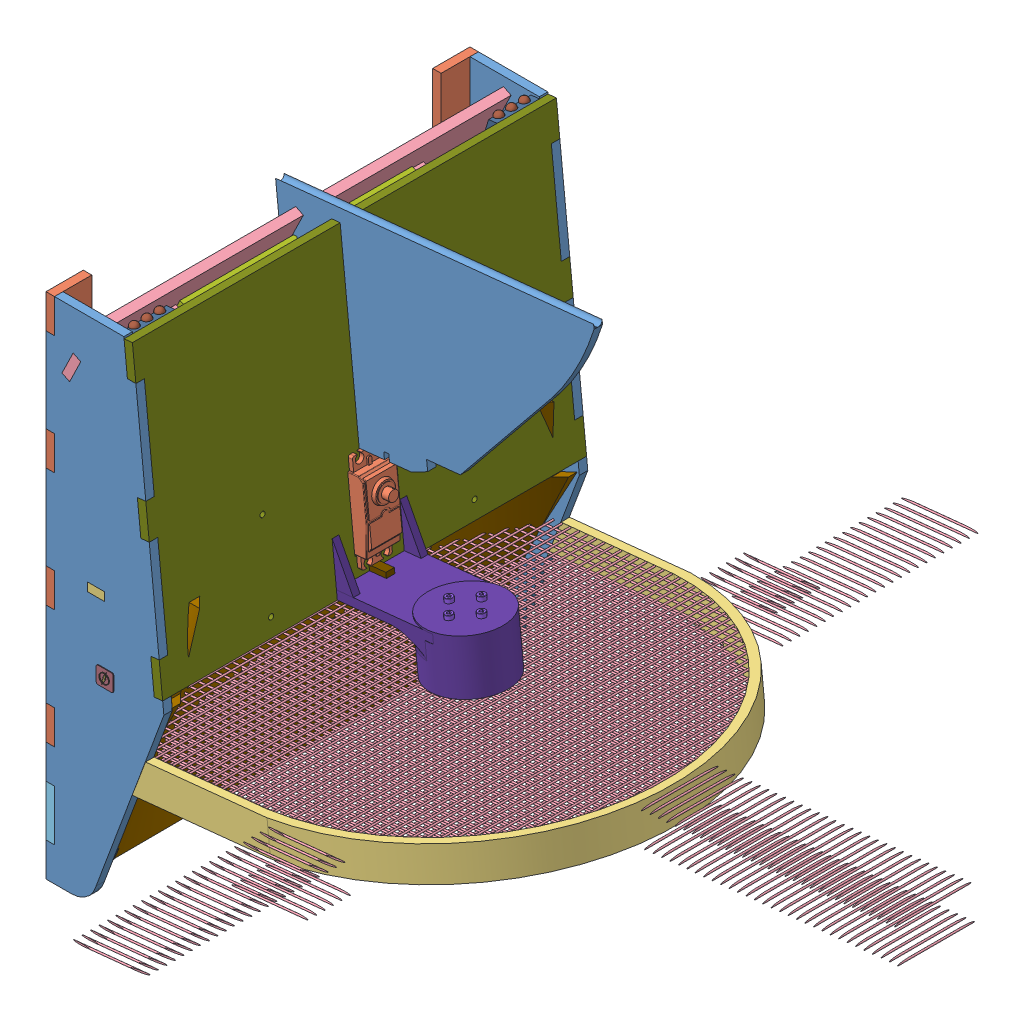
SolidWorks assembly AssStructSimu, configuration Défaut. Lengths in mm. (continued)
Components (placement in the parent): (continued)
- AssCarte-1: AssCarte [Défaut] at (38.0121 147.1029 290.772) x (-0.101852 0.9948 0) z (0.9948 0.101852 0) size (66.52 130.57 98.72) (hidden) (continued)
  - carte_onduleur_v3-1: carte_onduleur_v3 [Défaut] at (-131.8199 12.0892 20.7912) size (66.52 130.57 82.34) (continued)
    - CARTE_CMD-1: CARTE_CMD [Défaut] at (25 57.2 0.803) size (60.1 130 26.71) (continued)
      - Open CASCADE STEP translator 6.8 1.20.1-1: Open CASCADE STEP translator 6.8 1.20.1 [Défaut] at origin size (60.1 130 26.71) (continued)
        - Body_1_4-1: Body_1_4 [Défaut] at (-55 5 12) size (60.1 130 26.71) (continued)
          - 175-1: 175 [Défaut] at (10 -21.7 0.803) x (0 -1 0) z (0 0 1) size (15 25.4 12.78) (continued)
            - =_[0_1_1_72]-1: =_[0_1_1_72] [Défaut] at origin size (15 25.4 12.78) (continued)
              - 173-1: 173 [Défaut] at (-1.4 -1 12) x (-1 0 0) z (0 1 0) size (15 12.78 25.4) (continued)
                - hole_plating_20-20: hole_plating_20 [Défaut] at (-1.5 -1.58 23.93) size (1.5 0.01 1.5)
                - Pin_Header_1x10_TH_Pitch_2.54mm_1-1: Pin_Header_1x10_TH_Pitch_2.54mm_1 [Défaut] at (-1.5 -1.5786 23.93) x (0 0 -1) z (0 -1 0) size (25.4 2.54 12.7)
                  - 124-1: 124 [Défaut] at origin size (25.4 2.54 2.8)
                    - =_[0_1_1_77]-1: =_[0_1_1_77] [Défaut] at origin
                    - =_[0_1_1_79]-1: =_[0_1_1_79] [Défaut] at origin
                    - =_[0_1_1_80]-1: =_[0_1_1_80] [Défaut] at origin
                    - =_[0_1_1_81]-1: =_[0_1_1_81] [Défaut] at origin
                    - =_[0_1_1_82]-1: =_[0_1_1_82] [Défaut] at origin
                    - =_[0_1_1_83]-1: =_[0_1_1_83] [Défaut] at origin
                    - =_[0_1_1_84]-1: =_[0_1_1_84] [Défaut] at origin
                    - =_[0_1_1_85]-1: =_[0_1_1_85] [Défaut] at origin
                    - =_[0_1_1_86]-1: =_[0_1_1_86] [Défaut] at origin
                    - =_[0_1_1_87]-1: =_[0_1_1_87] [Défaut] at origin
                  - 135-1: 135 [Défaut] at origin size (23.49 0.63 12.7)
                    - =_[0_1_1_88]-1: =_[0_1_1_88] [Défaut] at origin size (0.63 0.63 12.7)
                    - =_[0_1_1_90]-1: =_[0_1_1_90] [Défaut] at origin size (0.63 0.63 12.7)
                    - =_[0_1_1_91]-1: =_[0_1_1_91] [Défaut] at origin size (0.63 0.63 12.7)
                    - =_[0_1_1_92]-1: =_[0_1_1_92] [Défaut] at origin size (0.63 0.63 12.7)
                    - =_[0_1_1_93]-1: =_[0_1_1_93] [Défaut] at origin size (0.63 0.63 12.7)
                    - =_[0_1_1_94]-1: =_[0_1_1_94] [Défaut] at origin size (0.63 0.63 12.7)
                    - =_[0_1_1_95]-1: =_[0_1_1_95] [Défaut] at origin size (0.63 0.63 12.7)
                    - =_[0_1_1_96]-1: =_[0_1_1_96] [Défaut] at origin size (0.63 0.63 12.7)
                    - =_[0_1_1_97]-1: =_[0_1_1_97] [Défaut] at origin size (0.63 0.63 12.7)
                    - =_[0_1_1_98]-1: =_[0_1_1_98] [Défaut] at origin size (0.63 0.63 12.7)
                - MPU-9250_1-1: MPU-9250_1 [Défaut] at (-8 0.05 12.5) x (-1 0 0) z (0 1 0) size (3 3 1.05)
                - tantalum_10uF_1-1: tantalum_10uF_1 [Défaut] at (-13.167 0.1 10.9372) x (0 0 1) z (0 1 0)
                - SOT23_5_1-1: SOT23_5_1 [Défaut] at (-7.475 -0.0136 21) x (0 0 1) z (0 1 0) size (3 3.2 0.92)
                - RESC-0603_5-1: RESC-0603_5 [Défaut] at (-6.85 0 7.45) x (1 0 0) z (0 1 0) size (1.7 0.9 0.55)
                  - 143-1: 143 [Défaut] at origin size (1.7 0.9 0.55)
                    - =_[0_1_1_103]-1: =_[0_1_1_103] [Défaut] at origin size (0.4 0.9 0.53)
                    - =_[0_1_1_105]-1: =_[0_1_1_105] [Défaut] at origin size (0.4 0.9 0.53)
                    - =_[0_1_1_106]-1: =_[0_1_1_106] [Défaut] at origin size (1.64 0.9 0.52)
                  - 152-1: 152 [Défaut] at origin
                    - =_[0_1_1_107]-1: =_[0_1_1_107] [Défaut] at origin
                    - =_[0_1_1_109]-1: =_[0_1_1_109] [Défaut] at origin
                    - =_[0_1_1_110]-1: =_[0_1_1_110] [Défaut] at origin
                    - =_[0_1_1_111]-1: =_[0_1_1_111] [Défaut] at origin
                    - =_[0_1_1_112]-1: =_[0_1_1_112] [Défaut] at origin
                    - =_[0_1_1_113]-1: =_[0_1_1_113] [Défaut] at origin
                    - =_[0_1_1_114]-1: =_[0_1_1_114] [Défaut] at origin
                    - =_[0_1_1_115]-1: =_[0_1_1_115] [Défaut] at origin
                - RESC-0603_5-2: RESC-0603_5 [Défaut] at (-9.85 0 16.05) x (1 0 0) z (0 1 0) size (1.7 0.9 0.55)
                  - 143-1: 143 [Défaut] at origin size (1.7 0.9 0.55)
                    - =_[0_1_1_103]-1: =_[0_1_1_103] [Défaut] at origin size (0.4 0.9 0.53)
                    - =_[0_1_1_105]-1: =_[0_1_1_105] [Défaut] at origin size (0.4 0.9 0.53)
                    - =_[0_1_1_106]-1: =_[0_1_1_106] [Défaut] at origin size (1.64 0.9 0.52)
                  - 152-1: 152 [Défaut] at origin
                    - =_[0_1_1_107]-1: =_[0_1_1_107] [Défaut] at origin
                    - =_[0_1_1_109]-1: =_[0_1_1_109] [Défaut] at origin
                    - =_[0_1_1_110]-1: =_[0_1_1_110] [Défaut] at origin
                    - =_[0_1_1_111]-1: =_[0_1_1_111] [Défaut] at origin
                    - =_[0_1_1_112]-1: =_[0_1_1_112] [Défaut] at origin
                    - =_[0_1_1_113]-1: =_[0_1_1_113] [Défaut] at origin
                    - =_[0_1_1_114]-1: =_[0_1_1_114] [Défaut] at origin
                    - =_[0_1_1_115]-1: =_[0_1_1_115] [Défaut] at origin
                - RESC-0603_5-3: RESC-0603_5 [Défaut] at (-6.85 0 17.55) x (1 0 0) z (0 1 0) size (1.7 0.9 0.55)
                  - 143-1: 143 [Défaut] at origin size (1.7 0.9 0.55)
                    - =_[0_1_1_103]-1: =_[0_1_1_103] [Défaut] at origin size (0.4 0.9 0.53)
                    - =_[0_1_1_105]-1: =_[0_1_1_105] [Défaut] at origin size (0.4 0.9 0.53)
                    - =_[0_1_1_106]-1: =_[0_1_1_106] [Défaut] at origin size (1.64 0.9 0.52)
                  - 152-1: 152 [Défaut] at origin
                    - =_[0_1_1_107]-1: =_[0_1_1_107] [Défaut] at origin
                    - =_[0_1_1_109]-1: =_[0_1_1_109] [Défaut] at origin
                    - =_[0_1_1_110]-1: =_[0_1_1_110] [Défaut] at origin
                    - =_[0_1_1_111]-1: =_[0_1_1_111] [Défaut] at origin
                    - =_[0_1_1_112]-1: =_[0_1_1_112] [Défaut] at origin
                    - =_[0_1_1_113]-1: =_[0_1_1_113] [Défaut] at origin
                    - =_[0_1_1_114]-1: =_[0_1_1_114] [Défaut] at origin
                    - =_[0_1_1_115]-1: =_[0_1_1_115] [Défaut] at origin
                - RESC-0603_5-4: RESC-0603_5 [Défaut] at (-6.85 0 16.05) x (1 0 0) z (0 1 0) size (1.7 0.9 0.55)
                  - 143-1: 143 [Défaut] at origin size (1.7 0.9 0.55)
                    - =_[0_1_1_103]-1: =_[0_1_1_103] [Défaut] at origin size (0.4 0.9 0.53)
                    - =_[0_1_1_105]-1: =_[0_1_1_105] [Défaut] at origin size (0.4 0.9 0.53)
                    - =_[0_1_1_106]-1: =_[0_1_1_106] [Défaut] at origin size (1.64 0.9 0.52)
                  - 152-1: 152 [Défaut] at origin
                    - =_[0_1_1_107]-1: =_[0_1_1_107] [Défaut] at origin
                    - =_[0_1_1_109]-1: =_[0_1_1_109] [Défaut] at origin
                    - =_[0_1_1_110]-1: =_[0_1_1_110] [Défaut] at origin
                    - =_[0_1_1_111]-1: =_[0_1_1_111] [Défaut] at origin
                    - =_[0_1_1_112]-1: =_[0_1_1_112] [Défaut] at origin
                    - =_[0_1_1_113]-1: =_[0_1_1_113] [Défaut] at origin
                    - =_[0_1_1_114]-1: =_[0_1_1_114] [Défaut] at origin
                    - =_[0_1_1_115]-1: =_[0_1_1_115] [Défaut] at origin
                - RESC-0603_5-5: RESC-0603_5 [Défaut] at (-6.85 0 5.95) x (1 0 0) z (0 1 0) size (1.7 0.9 0.55)
                  - 143-1: 143 [Défaut] at origin size (1.7 0.9 0.55)
                    - =_[0_1_1_103]-1: =_[0_1_1_103] [Défaut] at origin size (0.4 0.9 0.53)
                    - =_[0_1_1_105]-1: =_[0_1_1_105] [Défaut] at origin size (0.4 0.9 0.53)
                    - =_[0_1_1_106]-1: =_[0_1_1_106] [Défaut] at origin size (1.64 0.9 0.52)
                  - 152-1: 152 [Défaut] at origin
                    - =_[0_1_1_107]-1: =_[0_1_1_107] [Défaut] at origin
                    - =_[0_1_1_109]-1: =_[0_1_1_109] [Défaut] at origin
                    - =_[0_1_1_110]-1: =_[0_1_1_110] [Défaut] at origin
                    - =_[0_1_1_111]-1: =_[0_1_1_111] [Défaut] at origin
                    - =_[0_1_1_112]-1: =_[0_1_1_112] [Défaut] at origin
                    - =_[0_1_1_113]-1: =_[0_1_1_113] [Défaut] at origin
                    - =_[0_1_1_114]-1: =_[0_1_1_114] [Défaut] at origin
                    - =_[0_1_1_115]-1: =_[0_1_1_115] [Défaut] at origin
                - CAPC-0603-T0.9-BN_5-1: CAPC-0603-T0.9-BN_5 [Défaut] at (-9.85 0 8.95) x (1 0 0) z (0 1 0) size (1.7 0.9 0.9)
                  - =_[0_1_1_117]-1: =_[0_1_1_117] [Défaut] at origin size (1.7 0.9 0.9)
                  - 167-1: 167 [Défaut] at origin
                    - =_[0_1_1_118]-1: =_[0_1_1_118] [Défaut] at origin
                    - =_[0_1_1_120]-1: =_[0_1_1_120] [Défaut] at origin
                    - =_[0_1_1_121]-1: =_[0_1_1_121] [Défaut] at origin
                    - =_[0_1_1_122]-1: =_[0_1_1_122] [Défaut] at origin
                    - =_[0_1_1_123]-1: =_[0_1_1_123] [Défaut] at origin
                    - =_[0_1_1_124]-1: =_[0_1_1_124] [Défaut] at origin
                    - =_[0_1_1_125]-1: =_[0_1_1_125] [Défaut] at origin
                    - =_[0_1_1_126]-1: =_[0_1_1_126] [Défaut] at origin
                - CAPC-0603-T0.9-BN_5-2: CAPC-0603-T0.9-BN_5 [Défaut] at (-6.85 0 8.95) x (1 0 0) z (0 1 0) size (1.7 0.9 0.9)
                  - =_[0_1_1_117]-1: =_[0_1_1_117] [Défaut] at origin size (1.7 0.9 0.9)
                  - 167-1: 167 [Défaut] at origin
                    - =_[0_1_1_118]-1: =_[0_1_1_118] [Défaut] at origin
                    - =_[0_1_1_120]-1: =_[0_1_1_120] [Défaut] at origin
                    - =_[0_1_1_121]-1: =_[0_1_1_121] [Défaut] at origin
                    - =_[0_1_1_122]-1: =_[0_1_1_122] [Défaut] at origin
                    - =_[0_1_1_123]-1: =_[0_1_1_123] [Défaut] at origin
                    - =_[0_1_1_124]-1: =_[0_1_1_124] [Défaut] at origin
                    - =_[0_1_1_125]-1: =_[0_1_1_125] [Défaut] at origin
                    - =_[0_1_1_126]-1: =_[0_1_1_126] [Défaut] at origin
                - CAPC-0603-T0.9-BN_5-3: CAPC-0603-T0.9-BN_5 [Défaut] at (-6.85 0 19.05) x (1 0 0) z (0 1 0) size (1.7 0.9 0.9)
                  - =_[0_1_1_117]-1: =_[0_1_1_117] [Défaut] at origin size (1.7 0.9 0.9)
                  - 167-1: 167 [Défaut] at origin
                    - =_[0_1_1_118]-1: =_[0_1_1_118] [Défaut] at origin
                    - =_[0_1_1_120]-1: =_[0_1_1_120] [Défaut] at origin
                    - =_[0_1_1_121]-1: =_[0_1_1_121] [Défaut] at origin
                    - =_[0_1_1_122]-1: =_[0_1_1_122] [Défaut] at origin
                    - =_[0_1_1_123]-1: =_[0_1_1_123] [Défaut] at origin
                    - =_[0_1_1_124]-1: =_[0_1_1_124] [Défaut] at origin
                    - =_[0_1_1_125]-1: =_[0_1_1_125] [Défaut] at origin
                    - =_[0_1_1_126]-1: =_[0_1_1_126] [Défaut] at origin
                - CAPC-0603-T0.9-BN_5-4: CAPC-0603-T0.9-BN_5 [Défaut] at (-9.85 0 7.45) x (1 0 0) z (0 1 0) size (1.7 0.9 0.9)
                  - =_[0_1_1_117]-1: =_[0_1_1_117] [Défaut] at origin size (1.7 0.9 0.9)
                  - 167-1: 167 [Défaut] at origin
                    - =_[0_1_1_118]-1: =_[0_1_1_118] [Défaut] at origin
                    - =_[0_1_1_120]-1: =_[0_1_1_120] [Défaut] at origin
                    - =_[0_1_1_121]-1: =_[0_1_1_121] [Défaut] at origin
                    - =_[0_1_1_122]-1: =_[0_1_1_122] [Défaut] at origin
                    - =_[0_1_1_123]-1: =_[0_1_1_123] [Défaut] at origin
                    - =_[0_1_1_124]-1: =_[0_1_1_124] [Défaut] at origin
                    - =_[0_1_1_125]-1: =_[0_1_1_125] [Défaut] at origin
                    - =_[0_1_1_126]-1: =_[0_1_1_126] [Défaut] at origin
                - CAPC-0603-T0.9-BN_5-5: CAPC-0603-T0.9-BN_5 [Défaut] at (-9.85 0 17.55) x (1 0 0) z (0 1 0) size (1.7 0.9 0.9)
                  - =_[0_1_1_117]-1: =_[0_1_1_117] [Défaut] at origin size (1.7 0.9 0.9)
                  - 167-1: 167 [Défaut] at origin
                    - =_[0_1_1_118]-1: =_[0_1_1_118] [Défaut] at origin
                    - =_[0_1_1_120]-1: =_[0_1_1_120] [Défaut] at origin
                    - =_[0_1_1_121]-1: =_[0_1_1_121] [Défaut] at origin
                    - =_[0_1_1_122]-1: =_[0_1_1_122] [Défaut] at origin
                    - =_[0_1_1_123]-1: =_[0_1_1_123] [Défaut] at origin
                    - =_[0_1_1_124]-1: =_[0_1_1_124] [Défaut] at origin
                    - =_[0_1_1_125]-1: =_[0_1_1_125] [Défaut] at origin
                    - =_[0_1_1_126]-1: =_[0_1_1_126] [Défaut] at origin
          - 177-1: 177 [Défaut] at (52.1 -16.5 -0.803) x (1 0 0) z (0 0 -1) size (2.34 1.04 0.5)
            - =_[0_1_1_30]-1: =_[0_1_1_30] [Défaut] at origin size (2.34 1.04 0.5)
              - 32_2-1: 32_2 [Défaut] at origin size (2.29 1.04 0.43)
              - 33_2-1: 33_2 [Défaut] at (0.3048 0 0) x (-1 0 0) z (0 0 1) size (0.51 1.02 0.5)
              - 34-1: 34 [Défaut] at origin size (0.51 1.02 0.5)
          - 179-1: 179 [Défaut] at (22.5336 -121.5 -0.803) x (-1 0 0) z (0 0 -1) size (2.34 1.04 0.5)
            - =_[0_1_1_30]-1: =_[0_1_1_30] [Défaut] at origin size (2.34 1.04 0.5)
              - 32_2-1: 32_2 [Défaut] at origin size (2.29 1.04 0.43)
              - 33_2-1: 33_2 [Défaut] at (0.3048 0 0) x (-1 0 0) z (0 0 1) size (0.51 1.02 0.5)
              - 34-1: 34 [Défaut] at origin size (0.51 1.02 0.5)
          - 181-1: 181 [Défaut] at (48.6 -127 -0.803) x (-1 0 0) z (0 0 -1) size (2.34 1.04 0.5)
            - =_[0_1_1_30]-1: =_[0_1_1_30] [Défaut] at origin size (2.34 1.04 0.5)
              - 32_2-1: 32_2 [Défaut] at origin size (2.29 1.04 0.43)
              - 33_2-1: 33_2 [Défaut] at (0.3048 0 0) x (-1 0 0) z (0 0 1) size (0.51 1.02 0.5)
              - 34-1: 34 [Défaut] at origin size (0.51 1.02 0.5)
          - 183-1: 183 [Défaut] at (26.0189 -121.5 0.803) size (2.34 1.04 0.5)
            - =_[0_1_1_30]-1: =_[0_1_1_30] [Défaut] at origin size (2.34 1.04 0.5)
              - 32_2-1: 32_2 [Défaut] at origin size (2.29 1.04 0.43)
              - 33_2-1: 33_2 [Défaut] at (0.3048 0 0) x (-1 0 0) z (0 0 1) size (0.51 1.02 0.5)
              - 34-1: 34 [Défaut] at origin size (0.51 1.02 0.5)
          - 185-1: 185 [Défaut] at (30.3664 -19 -0.803) x (1 0 0) z (0 0 -1) size (2.34 1.04 0.5)
            - =_[0_1_1_30]-1: =_[0_1_1_30] [Défaut] at origin size (2.34 1.04 0.5)
              - 32_2-1: 32_2 [Défaut] at origin size (2.29 1.04 0.43)
              - 33_2-1: 33_2 [Défaut] at (0.3048 0 0) x (-1 0 0) z (0 0 1) size (0.51 1.02 0.5)
              - 34-1: 34 [Défaut] at origin size (0.51 1.02 0.5)
          - 187-1: 187 [Défaut] at (51.7 -114.3 -0.803) x (0 1 0) z (0 0 -1) size (2.34 1.04 0.5)
            - =_[0_1_1_30]-1: =_[0_1_1_30] [Défaut] at origin size (2.34 1.04 0.5)
              - 32_2-1: 32_2 [Défaut] at origin size (2.29 1.04 0.43)
              - 33_2-1: 33_2 [Défaut] at (0.3048 0 0) x (-1 0 0) z (0 0 1) size (0.51 1.02 0.5)
              - 34-1: 34 [Défaut] at origin size (0.51 1.02 0.5)
          - 189-1: 189 [Défaut] at (50 -114.3 -0.803) x (0 1 0) z (0 0 -1) size (2.34 1.04 0.5)
            - =_[0_1_1_30]-1: =_[0_1_1_30] [Défaut] at origin size (2.34 1.04 0.5)
              - 32_2-1: 32_2 [Défaut] at origin size (2.29 1.04 0.43)
              - 33_2-1: 33_2 [Défaut] at (0.3048 0 0) x (-1 0 0) z (0 0 1) size (0.51 1.02 0.5)
              - 34-1: 34 [Défaut] at origin size (0.51 1.02 0.5)
    - C2_1-1: C2_1 [Défaut] at (-20.6984 1.8 -0.803) x (1 0 0) z (0 0 -1) size (2.34 1.04 0.5)
      - Open CASCADE STEP translator 6.8 1.6.1-1: Open CASCADE STEP translator 6.8 1.6.1 [Défaut] at origin size (2.34 1.04 0.5)
        - Body_1-1: Body_1 [Défaut] at origin size (2.29 1.04 0.43)
        - Pin_1-1: Pin_1 [Défaut] at (0.3048 0 0) x (-1 0 0) z (0 0 1) size (0.51 1.02 0.5)
        - Pin_2-1: Pin_2 [Défaut] at origin size (0.51 1.02 0.5)
    - C2_2-1: C2_2 [Défaut] at (-24.2 1.8 -0.803) x (1 0 0) z (0 0 -1) size (2.34 1.04 0.5)
      - Open CASCADE STEP translator 6.8 1.6.1-1: Open CASCADE STEP translator 6.8 1.6.1 [Défaut] at origin size (2.34 1.04 0.5)
        - Body_1-1: Body_1 [Défaut] at origin size (2.29 1.04 0.43)
        - Pin_1-1: Pin_1 [Défaut] at (0.3048 0 0) x (-1 0 0) z (0 0 1) size (0.51 1.02 0.5)
        - Pin_2-1: Pin_2 [Défaut] at origin size (0.51 1.02 0.5)
    - C3_1-1: C3_1 [Défaut] at (-20.9176 -12.8 -0.803) x (1 0 0) z (0 0 -1) size (2.34 1.04 0.5)
      - Open CASCADE STEP translator 6.8 1.6.1-1: Open CASCADE STEP translator 6.8 1.6.1 [Défaut] at origin size (2.34 1.04 0.5)
        - Body_1-1: Body_1 [Défaut] at origin size (2.29 1.04 0.43)
        - Pin_1-1: Pin_1 [Défaut] at (0.3048 0 0) x (-1 0 0) z (0 0 1) size (0.51 1.02 0.5)
        - Pin_2-1: Pin_2 [Défaut] at origin size (0.51 1.02 0.5)
    - C3_2-1: C3_2 [Défaut] at (-24.4 -12.8 -0.803) x (1 0 0) z (0 0 -1) size (2.34 1.04 0.5)
      - Open CASCADE STEP translator 6.8 1.6.1-1: Open CASCADE STEP translator 6.8 1.6.1 [Défaut] at origin size (2.34 1.04 0.5)
        - Body_1-1: Body_1 [Défaut] at origin size (2.29 1.04 0.43)
        - Pin_1-1: Pin_1 [Défaut] at (0.3048 0 0) x (-1 0 0) z (0 0 1) size (0.51 1.02 0.5)
        - Pin_2-1: Pin_2 [Défaut] at origin size (0.51 1.02 0.5)
    - D_CUR-1: D_CUR [Défaut] at (-12.4432 3.85 -0.803) x (0 -1 0) z (0 0 -1) size (2.7 5.2 1.11)
      - Open CASCADE STEP translator 6.8 1.25.1-1: Open CASCADE STEP translator 6.8 1.25.1 [Défaut] at origin size (2.7 5.2 1.11)
        - Body_1_5-1: Body_1_5 [Défaut] at (1.2 -4 0) x (0 1 0) z (0 0 1) size (5.2 2.7 1.11)
          - =_[0_1_1_3]_4-1: =_[0_1_1_3]_4 [Défaut] at origin size (0.39 0.64 0.01)
          - =_[0_1_1_4]_4-1: =_[0_1_1_4]_4 [Défaut] at origin size (0.6 1.9 0.2)
          - =_[0_1_1_5]_4-1: =_[0_1_1_5]_4 [Défaut] at origin size (0.21 0.08 0.01)
          - =_[0_1_1_6]_2-1: =_[0_1_1_6]_2 [Défaut] at origin size (0.6 1.9 0.2)
          - =_[0_1_1_7]_2-1: =_[0_1_1_7]_2 [Défaut] at origin size (0.46 0.68 0.01)
          - =_[0_1_1_8]_2-1: =_[0_1_1_8]_2 [Défaut] at origin size (0.38 0.66 0.01)
          - =_[0_1_1_9]-1: =_[0_1_1_9] [Défaut] at origin size (0.2 0.62 0.01)
          - =_[0_1_1_10]-1: =_[0_1_1_10] [Défaut] at origin size (4 2.7 1.1)
          - =_[0_1_1_11]-1: =_[0_1_1_11] [Défaut] at origin size (0.46 0.63 0.01)
          - =_[0_1_1_12]-1: =_[0_1_1_12] [Défaut] at origin size (0.56 0.68 0.01)
    - RC1_1-1: RC1_1 [Défaut] at (-20.7176 8.1 -0.803) x (1 0 0) z (0 0 -1) size (2.34 1.04 0.5)
      - Open CASCADE STEP translator 6.8 1.12.1-1: Open CASCADE STEP translator 6.8 1.12.1 [Défaut] at origin size (2.34 1.04 0.5)
        - Body_1_3-1: Body_1_3 [Défaut] at origin size (2.29 1.04 0.43)
        - Pin_1_2-1: Pin_1_2 [Défaut] at (0.3048 0 0) x (-1 0 0) z (0 0 1) size (0.51 1.02 0.5)
        - Pin_2_2-1: Pin_2_2 [Défaut] at origin size (0.51 1.02 0.5)
    - RC1_2-1: RC1_2 [Défaut] at (-22 8.1 -0.803) x (-1 0 0) z (0 0 -1) size (2.34 1.04 0.5)
      - Open CASCADE STEP translator 6.8 1.12.1-1: Open CASCADE STEP translator 6.8 1.12.1 [Défaut] at origin size (2.34 1.04 0.5)
        - Body_1_3-1: Body_1_3 [Défaut] at origin size (2.29 1.04 0.43)
        - Pin_1_2-1: Pin_1_2 [Défaut] at (0.3048 0 0) x (-1 0 0) z (0 0 1) size (0.51 1.02 0.5)
        - Pin_2_2-1: Pin_2_2 [Défaut] at origin size (0.51 1.02 0.5)
    - RC2_1-1: RC2_1 [Défaut] at (-20.716 0.243 -0.803) x (1 0 0) z (0 0 -1) size (2.34 1.04 0.5)
      - Open CASCADE STEP translator 6.8 1.12.1-1: Open CASCADE STEP translator 6.8 1.12.1 [Défaut] at origin size (2.34 1.04 0.5)
        - Body_1_3-1: Body_1_3 [Défaut] at origin size (2.29 1.04 0.43)
        - Pin_1_2-1: Pin_1_2 [Défaut] at (0.3048 0 0) x (-1 0 0) z (0 0 1) size (0.51 1.02 0.5)
        - Pin_2_2-1: Pin_2_2 [Défaut] at origin size (0.51 1.02 0.5)
    - RC2_2-1: RC2_2 [Défaut] at (-22 0.18 -0.803) x (-1 0 0) z (0 0 -1) size (2.34 1.04 0.5)
      - Open CASCADE STEP translator 6.8 1.12.1-1: Open CASCADE STEP translator 6.8 1.12.1 [Défaut] at origin size (2.34 1.04 0.5)
        - Body_1_3-1: Body_1_3 [Défaut] at origin size (2.29 1.04 0.43)
        - Pin_1_2-1: Pin_1_2 [Défaut] at (0.3048 0 0) x (-1 0 0) z (0 0 1) size (0.51 1.02 0.5)
        - Pin_2_2-1: Pin_2_2 [Défaut] at origin size (0.51 1.02 0.5)
    - RC3_1-1: RC3_1 [Défaut] at (-20.9336 -14.5 -0.803) x (1 0 0) z (0 0 -1) size (2.34 1.04 0.5)
      - Open CASCADE STEP translator 6.8 1.12.1-1: Open CASCADE STEP translator 6.8 1.12.1 [Défaut] at origin size (2.34 1.04 0.5)
        - Body_1_3-1: Body_1_3 [Défaut] at origin size (2.29 1.04 0.43)
        - Pin_1_2-1: Pin_1_2 [Défaut] at (0.3048 0 0) x (-1 0 0) z (0 0 1) size (0.51 1.02 0.5)
        - Pin_2_2-1: Pin_2_2 [Défaut] at origin size (0.51 1.02 0.5)
    - RC3_2-1: RC3_2 [Défaut] at (-22.3 -14.5 -0.803) x (-1 0 0) z (0 0 -1) size (2.34 1.04 0.5)
      - Open CASCADE STEP translator 6.8 1.12.1-1: Open CASCADE STEP translator 6.8 1.12.1 [Défaut] at origin size (2.34 1.04 0.5)
        - Body_1_3-1: Body_1_3 [Défaut] at origin size (2.29 1.04 0.43)
        - Pin_1_2-1: Pin_1_2 [Défaut] at (0.3048 0 0) x (-1 0 0) z (0 0 1) size (0.51 1.02 0.5)
        - Pin_2_2-1: Pin_2_2 [Défaut] at origin size (0.51 1.02 0.5)
    - U_MES_CUR-1: U_MES_CUR [Défaut] at (-11.5 6.7816 0.803) size (2.54 2.41 0.76)
      - Open CASCADE STEP translator 6.8 1.32.1-1: Open CASCADE STEP translator 6.8 1.32.1 [Défaut] at origin size (2.54 2.41 0.76)
        - Body_1_5-1: Body_1_5 [Défaut] at origin size (2.54 1.27 0.71)
        - Pin_1_3-1: Pin_1_3 [Défaut] at (-2.1082 0.2286 0) x (0 -1 0) z (0 0 1) size (1.14 0.25 0.47)
        - Pin_2_3-1: Pin_2_3 [Défaut] at (-0.2032 2.1336 0) x (0 -1 0) z (0 0 1) size (1.14 0.25 0.47)
    - CARTE_ALIM-1: CARTE_ALIM [Défaut] at (-6.4 -57.2 0.803) size (60 130 18.35)
      - Open CASCADE STEP translator 6.8 1.33.1-1: Open CASCADE STEP translator 6.8 1.33.1 [Défaut] at origin size (60 130 18.35)
        - Body_1_6-1: Body_1_6 [Défaut] at (7 56 -12) size (60 130 18.35)
          - 1_3-1: 1_3 [Défaut] at origin size (60 130 1.61)
          - 13_3-1: 13_3 [Défaut] at (0.4717 -40.93 0.803) x (0 1 0) z (0 0 1) size (5.65 4.9 1.7)
            - =_[0_1_1_4]_3-1: =_[0_1_1_4]_3 [Défaut] at origin size (5.65 4.9 1.7)
              - 2-1: 2 [Défaut] at origin size (3.75 4.9 1.53)
              - 3-1: 3 [Défaut] at origin size (0.95 0.51 1.06)
              - 4-1: 4 [Défaut] at origin size (0.95 0.51 1.06)
              - 5_2-1: 5_2 [Défaut] at origin size (0.95 0.51 1.06)
              - 6-1: 6 [Défaut] at origin size (0.95 0.51 1.06)
              - 7-1: 7 [Défaut] at (10.8 -5.08 0) x (-1 0 0) z (0 0 1) size (0.95 0.51 1.06)
              - 8_2-1: 8_2 [Défaut] at (10.8 -2.54 0) x (-1 0 0) z (0 0 1) size (0.95 0.51 1.06)
              - 9-1: 9 [Défaut] at (10.8 0 0) x (-1 0 0) z (0 0 1) size (0.95 0.51 1.06)
              - 10-1: 10 [Défaut] at (10.8 2.54 0) x (-1 0 0) z (0 0 1) size (0.95 0.51 1.06)
              - 11_2-1: 11_2 [Défaut] at (5.4 -1.27 0) x (-1 0 0) z (0 0 1) size (4.25 2.34 1.06)
          - 18-1: 18 [Défaut] at (-2.5283 -37.23 0.803) x (0 -1 0) z (0 0 1) size (2.34 1.04 0.5)
            - =_[0_1_1_16]-1: =_[0_1_1_16] [Défaut] at origin size (2.34 1.04 0.5)
              - 14_2-1: 14_2 [Défaut] at origin size (2.29 1.04 0.43)
              - 15_2-1: 15_2 [Défaut] at (0.3048 0 0) x (-1 0 0) z (0 0 1) size (0.51 1.02 0.5)
              - 16_2-1: 16_2 [Défaut] at origin size (0.51 1.02 0.5)
          - 21_2-1: 21_2 [Défaut] at (-2.2263 -24.628 -0.803) x (1 0 0) z (0 0 -1) size (8.01 8 14.24)
            - =_[0_1_1_21]-1: =_[0_1_1_21] [Défaut] at origin size (8.01 8 14.24)
              - 19-1: 19 [Défaut] at (1.8 0 0) x (1 0 0) z (0 -1 0) size (8.01 14.24 8)
          - 23_2-1: 23_2 [Défaut] at (1.2381 -31.53 0.803) size (2.34 1.04 0.5)
            - =_[0_1_1_16]-1: =_[0_1_1_16] [Défaut] at origin size (2.34 1.04 0.5)
              - 14_2-1: 14_2 [Défaut] at origin size (2.29 1.04 0.43)
              - 15_2-1: 15_2 [Défaut] at (0.3048 0 0) x (-1 0 0) z (0 0 1) size (0.51 1.02 0.5)
              - 16_2-1: 16_2 [Défaut] at origin size (0.51 1.02 0.5)
          - 28-1: 28 [Défaut] at (5 29.8636 0.803) x (0 -1 0) z (0 0 1) size (3.35 1.3 0.55)
            - =_[0_1_1_25]_2-1: =_[0_1_1_25]_2 [Défaut] at origin size (3.35 1.3 0.55)
              - 24-1: 24 [Défaut] at origin size (3.3 1.3 0.48)
              - 25_2-1: 25_2 [Défaut] at (0.5588 0 0) x (-1 0 0) z (0 0 1) size (0.76 1.27 0.55)
              - 26_2-1: 26_2 [Défaut] at origin size (0.76 1.27 0.55)
          - 30-1: 30 [Défaut] at (6.7 29.8636 0.803) x (0 -1 0) z (0 0 1) size (2.34 1.04 0.5)
            - =_[0_1_1_16]-1: =_[0_1_1_16] [Défaut] at origin size (2.34 1.04 0.5)
              - 14_2-1: 14_2 [Défaut] at origin size (2.29 1.04 0.43)
              - 15_2-1: 15_2 [Défaut] at (0.3048 0 0) x (-1 0 0) z (0 0 1) size (0.51 1.02 0.5)
              - 16_2-1: 16_2 [Défaut] at origin size (0.51 1.02 0.5)
          - 35_2-1: 35_2 [Défaut] at (-2.5 -46.37 0.803) x (0 1 0) z (0 0 1) size (3.4 2.06 0.79)
            - =_[0_1_1_31]-1: =_[0_1_1_31] [Défaut] at origin size (3.4 2.06 0.79)
              - 31_2-1: 31_2 [Défaut] at origin size (3.3 2.06 0.69)
              - 32_3-1: 32_3 [Défaut] at (0.5588 0 0) x (-1 0 0) z (0 0 1) size (0.81 2.03 0.79)
              - 33_3-1: 33_3 [Défaut] at origin size (0.81 2.03 0.79)
          - 37-1: 37 [Défaut] at (5 31.43 0.803) x (0 1 0) z (0 0 1) size (2.34 1.04 0.5)
            - =_[0_1_1_16]-1: =_[0_1_1_16] [Défaut] at origin size (2.34 1.04 0.5)
              - 14_2-1: 14_2 [Défaut] at origin size (2.29 1.04 0.43)
              - 15_2-1: 15_2 [Défaut] at (0.3048 0 0) x (-1 0 0) z (0 0 1) size (0.51 1.02 0.5)
              - 16_2-1: 16_2 [Défaut] at origin size (0.51 1.02 0.5)
          - 39-1: 39 [Défaut] at (-0.2 35.63 0.803) x (-1 0 0) z (0 0 1) size (2.34 1.04 0.5)
            - =_[0_1_1_16]-1: =_[0_1_1_16] [Défaut] at origin size (2.34 1.04 0.5)
              - 14_2-1: 14_2 [Défaut] at origin size (2.29 1.04 0.43)
              - 15_2-1: 15_2 [Défaut] at (0.3048 0 0) x (-1 0 0) z (0 0 1) size (0.51 1.02 0.5)
              - 16_2-1: 16_2 [Défaut] at origin size (0.51 1.02 0.5)
          - 41-1: 41 [Défaut] at (2.9 -45.5036 0.803) x (0 1 0) z (0 0 1) size (2.34 1.04 0.5)
            - =_[0_1_1_16]-1: =_[0_1_1_16] [Défaut] at origin size (2.34 1.04 0.5)
              - 14_2-1: 14_2 [Défaut] at origin size (2.29 1.04 0.43)
              - 15_2-1: 15_2 [Défaut] at (0.3048 0 0) x (-1 0 0) z (0 0 1) size (0.51 1.02 0.5)
              - 16_2-1: 16_2 [Défaut] at origin size (0.51 1.02 0.5)
          - 43-1: 43 [Défaut] at (17.1348 -42.6272 0.803) x (0 1 0) z (0 0 1) size (2.34 1.04 0.5)
            - =_[0_1_1_16]-1: =_[0_1_1_16] [Défaut] at origin size (2.34 1.04 0.5)
              - 14_2-1: 14_2 [Défaut] at origin size (2.29 1.04 0.43)
              - 15_2-1: 15_2 [Défaut] at (0.3048 0 0) x (-1 0 0) z (0 0 1) size (0.51 1.02 0.5)
              - 16_2-1: 16_2 [Défaut] at origin size (0.51 1.02 0.5)
          - 48_2-1: 48_2 [Défaut] at (-5.4717 -39.01 0.803) x (-1 0 0) z (0 0 1) size (4.19 3.4 1.75)
            - =_[0_1_1_40]-1: =_[0_1_1_40] [Défaut] at origin size (4.19 3.4 1.75)
              - 44_2-1: 44_2 [Défaut] at origin size (3.75 3.38 1.73)
              - 45_2-1: 45_2 [Défaut] at (0.438 0 0) x (-1 0 0) z (0 0 1) size (0.53 3.4 1.75)
              - 46_2-1: 46_2 [Défaut] at origin size (0.52 3.4 1.75)
          - 53-1: 53 [Défaut] at (0.9 35.63 0.803) size (2.34 1.04 0.5)
            - =_[0_1_1_45]-1: =_[0_1_1_45] [Défaut] at origin size (2.34 1.04 0.5)
              - 49_3-1: 49_3 [Défaut] at origin size (2.29 1.04 0.43)
              - 50-1: 50 [Défaut] at (0.3048 0 0) x (-1 0 0) z (0 0 1) size (0.51 1.02 0.5)
              - 51-1: 51 [Défaut] at origin size (0.51 1.02 0.5)
          - 55_2-1: 55_2 [Défaut] at (1.3 -45.5036 0.803) x (0 1 0) z (0 0 1) size (2.34 1.04 0.5)
            - =_[0_1_1_45]-1: =_[0_1_1_45] [Défaut] at origin size (2.34 1.04 0.5)
              - 49_3-1: 49_3 [Défaut] at origin size (2.29 1.04 0.43)
              - 50-1: 50 [Défaut] at (0.3048 0 0) x (-1 0 0) z (0 0 1) size (0.51 1.02 0.5)
              - 51-1: 51 [Défaut] at origin size (0.51 1.02 0.5)
          - 57_3-1: 57_3 [Défaut] at (17.2348 -43.9936 0.803) x (0 -1 0) z (0 0 1) size (2.34 1.04 0.5)
            - =_[0_1_1_45]-1: =_[0_1_1_45] [Défaut] at origin size (2.34 1.04 0.5)
              - 49_3-1: 49_3 [Défaut] at origin size (2.29 1.04 0.43)
              - 50-1: 50 [Défaut] at (0.3048 0 0) x (-1 0 0) z (0 0 1) size (0.51 1.02 0.5)
              - 51-1: 51 [Défaut] at origin size (0.51 1.02 0.5)
          - 65-1: 65 [Défaut] at (-4.8 30.93 0.803) x (-1 0 0) z (0 0 1) size (14.64 9.83 4.25)
            - =_[0_1_1_52]-1: =_[0_1_1_52] [Défaut] at origin size (14.64 9.83 4.25)
              - 63_2-1: 63_2 [Défaut] at (3 0 0) x (0 -1 0) z (0 0 1) size (9.83 14.64 4.25)
                - =_[0_1_1_3]_5-1: =_[0_1_1_3]_5 [Défaut] at origin size (9.83 9.05 4.21)
                - =_[0_1_1_4]_5-1: =_[0_1_1_4]_5 [Défaut] at origin size (9.48 7.76 1.21)
                - =_[0_1_1_5]_5-1: =_[0_1_1_5]_5 [Défaut] at origin size (1.36 6.01 3.08)
                - =_[0_1_1_6]_3-1: =_[0_1_1_6]_3 [Défaut] at origin size (1.36 6.01 3.08)
                - =_[0_1_1_7]_3-1: =_[0_1_1_7]_3 [Défaut] at origin size (1.06 6.01 3.08)
          - 67-1: 67 [Défaut] at (13.5933 -37.5272 0.803) x (-1 0 0) z (0 0 1) size (2.34 1.04 0.5)
            - =_[0_1_1_16]-1: =_[0_1_1_16] [Défaut] at origin size (2.34 1.04 0.5)
              - 14_2-1: 14_2 [Défaut] at origin size (2.29 1.04 0.43)
              - 15_2-1: 15_2 [Défaut] at (0.3048 0 0) x (-1 0 0) z (0 0 1) size (0.51 1.02 0.5)
              - 16_2-1: 16_2 [Défaut] at origin size (0.51 1.02 0.5)
          - 70_2-1: 70_2 [Défaut] at (18.2733 -29.7272 0.803) x (0 1 0) z (0 0 1) size (6.06 4.95 1.88)
            - =_[0_1_1_61]-1: =_[0_1_1_61] [Défaut] at origin size (6.06 4.95 1.88)
              - 68-1: 68 [Défaut] x (1 0 0) z (0 -1 0) size (6.06 1.88 4.95)
          - 83-1: 83 [Défaut] at (-21.2 -38.07 0.803) x (-1 0 0) z (0 0 1) size (2.7 5.2 1.11)
            - =_[0_1_1_64]-1: =_[0_1_1_64] [Défaut] at origin size (2.7 5.2 1.11)
              - 84_2-1: 84_2 [Défaut] at (1.2 -4 0) x (0 1 0) z (0 0 1) size (5.2 2.7 1.11)
                - =_[0_1_1_3]_6-1: =_[0_1_1_3]_6 [Défaut] at origin size (0.39 0.64 0.01)
                - =_[0_1_1_4]_6-1: =_[0_1_1_4]_6 [Défaut] at origin size (0.6 1.9 0.2)
                - =_[0_1_1_5]_6-1: =_[0_1_1_5]_6 [Défaut] at origin size (0.21 0.08 0.01)
                - =_[0_1_1_6]_4-1: =_[0_1_1_6]_4 [Défaut] at origin size (0.6 1.9 0.2)
                - =_[0_1_1_7]_4-1: =_[0_1_1_7]_4 [Défaut] at origin size (0.46 0.68 0.01)
                - =_[0_1_1_8]_3-1: =_[0_1_1_8]_3 [Défaut] at origin size (0.38 0.66 0.01)
                - =_[0_1_1_9]_2-1: =_[0_1_1_9]_2 [Défaut] at origin size (0.2 0.62 0.01)
                - =_[0_1_1_10]_2-1: =_[0_1_1_10]_2 [Défaut] at origin size (4 2.7 1.1)
                - =_[0_1_1_11]_2-1: =_[0_1_1_11]_2 [Défaut] at origin size (0.46 0.63 0.01)
                - =_[0_1_1_12]_2-1: =_[0_1_1_12]_2 [Défaut] at origin size (0.56 0.68 0.01)
          - 86_2-1: 86_2 [Défaut] at (12.8933 -35.4272 0.803) x (0 1 0) z (0 0 1) size (2.7 5.2 1.11)
            - =_[0_1_1_77]-1: =_[0_1_1_77] [Défaut] at origin size (2.7 5.2 1.11)
              - 84_2-1: 84_2 [Défaut] at (1.2 -4 0) x (0 1 0) z (0 0 1) size (5.2 2.7 1.11)
                - =_[0_1_1_3]_6-1: =_[0_1_1_3]_6 [Défaut] at origin size (0.39 0.64 0.01)
                - =_[0_1_1_4]_6-1: =_[0_1_1_4]_6 [Défaut] at origin size (0.6 1.9 0.2)
                - =_[0_1_1_5]_6-1: =_[0_1_1_5]_6 [Défaut] at origin size (0.21 0.08 0.01)
                - =_[0_1_1_6]_4-1: =_[0_1_1_6]_4 [Défaut] at origin size (0.6 1.9 0.2)
                - =_[0_1_1_7]_4-1: =_[0_1_1_7]_4 [Défaut] at origin size (0.46 0.68 0.01)
                - =_[0_1_1_8]_3-1: =_[0_1_1_8]_3 [Défaut] at origin size (0.38 0.66 0.01)
                - =_[0_1_1_9]_2-1: =_[0_1_1_9]_2 [Défaut] at origin size (0.2 0.62 0.01)
                - =_[0_1_1_10]_2-1: =_[0_1_1_10]_2 [Défaut] at origin size (4 2.7 1.1)
                - =_[0_1_1_11]_2-1: =_[0_1_1_11]_2 [Défaut] at origin size (0.46 0.63 0.01)
                - =_[0_1_1_12]_2-1: =_[0_1_1_12]_2 [Défaut] at origin size (0.56 0.68 0.01)
          - 92_2-1: 92_2 [Défaut] at (20.9933 -39.3272 0.803) x (0 -1 0) z (0 0 1) size (2.79 1.98 0.64)
            - =_[0_1_1_79]-1: =_[0_1_1_79] [Défaut] at origin size (2.79 1.98 0.64)
              - 87-1: 87 [Défaut] at origin size (2.79 1.02 0.58)
              - 88-1: 88 [Défaut] x (0 -1 0) z (0 0 1) size (0.42 0.38 0.38)
              - 89-1: 89 [Défaut] at (-2.8448 -0.9652 0) x (0 1 0) z (0 0 1) size (0.55 0.38 0.38)
              - 90-1: 90 [Défaut] at (-0.9652 -2.8448 0) x (0 1 0) z (0 0 1) size (0.55 0.38 0.38)
          - 98-1: 98 [Défaut] at (-17.7 -48.47 0.803) x (0 -1 0) z (0 0 1) size (2.54 1.98 0.64)
            - =_[0_1_1_85]-1: =_[0_1_1_85] [Défaut] at origin size (2.54 1.98 0.64)
              - 93-1: 93 [Défaut] at origin size (2.54 1.14 0.58)
              - 94-1: 94 [Défaut] x (0 -1 0) z (0 0 1) size (0.43 0.51 0.38)
              - 95-1: 95 [Défaut] at (1.8796 1.8796 0) x (0 -1 0) z (0 0 1) size (0.43 0.51 0.38)
              - 96-1: 96 [Défaut] at (-0.9652 -2.8448 0) x (0 1 0) z (0 0 1) size (0.41 0.51 0.38)
          - 100-1: 100 [Défaut] at (24.3933 -43.2272 0.803) size (2.79 1.98 0.64)
            - =_[0_1_1_79]-1: =_[0_1_1_79] [Défaut] at origin size (2.79 1.98 0.64)
              - 87-1: 87 [Défaut] at origin size (2.79 1.02 0.58)
              - 88-1: 88 [Défaut] x (0 -1 0) z (0 0 1) size (0.42 0.38 0.38)
              - 89-1: 89 [Défaut] at (-2.8448 -0.9652 0) x (0 1 0) z (0 0 1) size (0.55 0.38 0.38)
              - 90-1: 90 [Défaut] at (-0.9652 -2.8448 0) x (0 1 0) z (0 0 1) size (0.55 0.38 0.38)
          - 102-1: 102 [Défaut] at (21.4933 -44.4272 0.803) x (0 -1 0) z (0 0 1) size (2.79 1.98 0.64)
            - =_[0_1_1_79]-1: =_[0_1_1_79] [Défaut] at origin size (2.79 1.98 0.64)
              - 87-1: 87 [Défaut] at origin size (2.79 1.02 0.58)
              - 88-1: 88 [Défaut] x (0 -1 0) z (0 0 1) size (0.42 0.38 0.38)
              - 89-1: 89 [Défaut] at (-2.8448 -0.9652 0) x (0 1 0) z (0 0 1) size (0.55 0.38 0.38)
              - 90-1: 90 [Défaut] at (-0.9652 -2.8448 0) x (0 1 0) z (0 0 1) size (0.55 0.38 0.38)
          - 107-1: 107 [Défaut] at (23.1933 -29.1272 -0.803) x (0 1 0) z (0 0 -1) size (9.6 14.35 5)
            - =_[0_1_1_93]-1: =_[0_1_1_93] [Défaut] at origin size (9.6 14.35 5)
              - 105-1: 105 [Défaut] at (0.5 -1 2) x (-1 0 0) z (0 0 1) size (9.6 14.35 5)
                - =_[0_1_1_3]_7-1: =_[0_1_1_3]_7 [Défaut] at origin size (9.6 12.75 5)
                - =_[0_1_1_4]_7-1: =_[0_1_1_4]_7 [Défaut] at origin size (2.2 1.6 2.2)
          - 109-1: 109 [Défaut] at (25.4933 -41.1272 0.803) x (-1 0 0) z (0 0 1) size (2.34 1.04 0.5)
            - =_[0_1_1_45]-1: =_[0_1_1_45] [Défaut] at origin size (2.34 1.04 0.5)
              - 49_3-1: 49_3 [Défaut] at origin size (2.29 1.04 0.43)
              - 50-1: 50 [Défaut] at (0.3048 0 0) x (-1 0 0) z (0 0 1) size (0.51 1.02 0.5)
              - 51-1: 51 [Défaut] at origin size (0.51 1.02 0.5)
          - 111-1: 111 [Défaut] at (22.0269 -41.8272 0.803) x (-1 0 0) z (0 0 1) size (2.34 1.04 0.5)
            - =_[0_1_1_45]-1: =_[0_1_1_45] [Défaut] at origin size (2.34 1.04 0.5)
              - 49_3-1: 49_3 [Défaut] at origin size (2.29 1.04 0.43)
              - 50-1: 50 [Défaut] at (0.3048 0 0) x (-1 0 0) z (0 0 1) size (0.51 1.02 0.5)
              - 51-1: 51 [Défaut] at origin size (0.51 1.02 0.5)
          - 113-1: 113 [Défaut] at (-24.8 -36.7036 0.803) x (0 1 0) z (0 0 1) size (2.34 1.04 0.5)
            - =_[0_1_1_45]-1: =_[0_1_1_45] [Défaut] at origin size (2.34 1.04 0.5)
              - 49_3-1: 49_3 [Défaut] at origin size (2.29 1.04 0.43)
              - 50-1: 50 [Défaut] at (0.3048 0 0) x (-1 0 0) z (0 0 1) size (0.51 1.02 0.5)
              - 51-1: 51 [Défaut] at origin size (0.51 1.02 0.5)
          - 115-1: 115 [Défaut] at (-24.8 -40.3036 0.803) x (0 1 0) z (0 0 1) size (2.34 1.04 0.5)
            - =_[0_1_1_45]-1: =_[0_1_1_45] [Défaut] at origin size (2.34 1.04 0.5)
              - 49_3-1: 49_3 [Défaut] at origin size (2.29 1.04 0.43)
              - 50-1: 50 [Défaut] at (0.3048 0 0) x (-1 0 0) z (0 0 1) size (0.51 1.02 0.5)
              - 51-1: 51 [Défaut] at origin size (0.51 1.02 0.5)
          - 117-1: 117 [Défaut] at (-16 -48.27 0.803) x (0 -1 0) z (0 0 1) size (2.34 1.04 0.5)
            - =_[0_1_1_45]-1: =_[0_1_1_45] [Défaut] at origin size (2.34 1.04 0.5)
              - 49_3-1: 49_3 [Défaut] at origin size (2.29 1.04 0.43)
              - 50-1: 50 [Défaut] at (0.3048 0 0) x (-1 0 0) z (0 0 1) size (0.51 1.02 0.5)
              - 51-1: 51 [Défaut] at origin size (0.51 1.02 0.5)
          - 119-1: 119 [Défaut] at (-22.5189 -47.87 0.803) x (-1 0 0) z (0 0 1) size (2.34 1.04 0.5)
            - =_[0_1_1_45]-1: =_[0_1_1_45] [Défaut] at origin size (2.34 1.04 0.5)
              - 49_3-1: 49_3 [Défaut] at origin size (2.29 1.04 0.43)
              - 50-1: 50 [Défaut] at (0.3048 0 0) x (-1 0 0) z (0 0 1) size (0.51 1.02 0.5)
              - 51-1: 51 [Défaut] at origin size (0.51 1.02 0.5)
          - 121-1: 121 [Défaut] at (22.3933 -38.9272 0.803) size (2.34 1.04 0.5)
            - =_[0_1_1_45]-1: =_[0_1_1_45] [Défaut] at origin size (2.34 1.04 0.5)
              - 49_3-1: 49_3 [Défaut] at origin size (2.29 1.04 0.43)
              - 50-1: 50 [Défaut] at (0.3048 0 0) x (-1 0 0) z (0 0 1) size (0.51 1.02 0.5)
              - 51-1: 51 [Défaut] at origin size (0.51 1.02 0.5)
          - 123-1: 123 [Défaut] at (22.0933 -36.4272 0.803) x (-1 0 0) z (0 0 1) size (2.34 1.04 0.5)
            - =_[0_1_1_45]-1: =_[0_1_1_45] [Défaut] at origin size (2.34 1.04 0.5)
              - 49_3-1: 49_3 [Défaut] at origin size (2.29 1.04 0.43)
              - 50-1: 50 [Défaut] at (0.3048 0 0) x (-1 0 0) z (0 0 1) size (0.51 1.02 0.5)
              - 51-1: 51 [Défaut] at origin size (0.51 1.02 0.5)
          - 125-1: 125 [Défaut] at (22.3933 -32.0272 0.803) x (0 -1 0) z (0 0 1) size (2.34 1.04 0.5)
            - =_[0_1_1_45]-1: =_[0_1_1_45] [Défaut] at origin size (2.34 1.04 0.5)
              - 49_3-1: 49_3 [Défaut] at origin size (2.29 1.04 0.43)
              - 50-1: 50 [Défaut] at (0.3048 0 0) x (-1 0 0) z (0 0 1) size (0.51 1.02 0.5)
              - 51-1: 51 [Défaut] at origin size (0.51 1.02 0.5)
          - 127-1: 127 [Défaut] at (17.9597 -23.1272 0.803) size (2.34 1.04 0.5)
            - =_[0_1_1_16]-1: =_[0_1_1_16] [Défaut] at origin size (2.34 1.04 0.5)
              - 14_2-1: 14_2 [Défaut] at origin size (2.29 1.04 0.43)
              - 15_2-1: 15_2 [Défaut] at (0.3048 0 0) x (-1 0 0) z (0 0 1) size (0.51 1.02 0.5)
              - 16_2-1: 16_2 [Défaut] at origin size (0.51 1.02 0.5)
          - 129-1: 129 [Défaut] at (20.0269 -24.9272 0.803) x (-1 0 0) z (0 0 1) size (2.34 1.04 0.5)
            - =_[0_1_1_16]-1: =_[0_1_1_16] [Défaut] at origin size (2.34 1.04 0.5)
              - 14_2-1: 14_2 [Défaut] at origin size (2.29 1.04 0.43)
              - 15_2-1: 15_2 [Défaut] at (0.3048 0 0) x (-1 0 0) z (0 0 1) size (0.51 1.02 0.5)
              - 16_2-1: 16_2 [Défaut] at origin size (0.51 1.02 0.5)
          - 131-1: 131 [Défaut] at (16.9933 -37.5272 0.803) x (-1 0 0) z (0 0 1) size (2.34 1.04 0.5)
            - =_[0_1_1_45]-1: =_[0_1_1_45] [Défaut] at origin size (2.34 1.04 0.5)
              - 49_3-1: 49_3 [Défaut] at origin size (2.29 1.04 0.43)
              - 50-1: 50 [Défaut] at (0.3048 0 0) x (-1 0 0) z (0 0 1) size (0.51 1.02 0.5)
              - 51-1: 51 [Défaut] at origin size (0.51 1.02 0.5)
          - 136-1: 136 [Défaut] at (3.2957 -29.23 0.803) x (-1 0 0) z (0 0 1) size (4.78 2.79 2.03)
            - =_[0_1_1_110]_2-1: =_[0_1_1_110]_2 [Défaut] at origin size (4.78 2.79 2.03)
              - 132-1: 132 [Défaut] at origin size (4.32 2.79 1.78)
              - 133-1: 133 [Défaut] at (0.4572 0 0) x (-1 0 0) z (0 0 1) size (1.02 1.27 1.32)
              - 134-1: 134 [Défaut] at origin size (1.02 1.27 1.32)
          - 141-1: 141 [Défaut] at (0.2436 -33.3673 0.803) size (3.35 1.3 0.55)
            - =_[0_1_1_115]_2-1: =_[0_1_1_115]_2 [Défaut] at origin size (3.35 1.3 0.55)
              - 137-1: 137 [Défaut] at origin size (3.3 1.3 0.48)
              - 138-1: 138 [Défaut] at (0.5588 0 0) x (-1 0 0) z (0 0 1) size (0.76 1.27 0.55)
              - 139-1: 139 [Défaut] at origin size (0.76 1.27 0.55)
          - 143_2-1: 143_2 [Défaut] at (-0.3 -45.47 0.803) x (0 1 0) z (0 0 1) size (2.34 1.04 0.5)
            - =_[0_1_1_16]-1: =_[0_1_1_16] [Défaut] at origin size (2.34 1.04 0.5)
              - 14_2-1: 14_2 [Défaut] at origin size (2.29 1.04 0.43)
              - 15_2-1: 15_2 [Défaut] at (0.3048 0 0) x (-1 0 0) z (0 0 1) size (0.51 1.02 0.5)
              - 16_2-1: 16_2 [Défaut] at origin size (0.51 1.02 0.5)
          - 145-1: 145 [Défaut] at (6.6 31.13 0.803) x (0 1 0) z (0 0 1) size (3.35 1.3 0.55)
            - =_[0_1_1_25]_2-1: =_[0_1_1_25]_2 [Défaut] at origin size (3.35 1.3 0.55)
              - 24-1: 24 [Défaut] at origin size (3.3 1.3 0.48)
              - 25_2-1: 25_2 [Défaut] at (0.5588 0 0) x (-1 0 0) z (0 0 1) size (0.76 1.27 0.55)
              - 26_2-1: 26_2 [Défaut] at origin size (0.76 1.27 0.55)
          - 148-1: 148 [Défaut] at (-7.5 -56.57 0.803) size (15.24 2.54 7.37)
            - =_[0_1_1_122]_2-1: =_[0_1_1_122]_2 [Défaut] at origin size (15.24 2.54 7.37)
              - 146-1: 146 [Défaut] at (6.3 0 1) x (1 0 0) z (0 -1 0) size (15.24 7.37 2.54)
    - COMP1-1: COMP1 [Défaut] at (-16.3 -36.2 0.803) x (-1 0 0) z (0 0 1) size (2.03 1.88 0.51)
      - Open CASCADE STEP translator 6.8 1.34.1-1: Open CASCADE STEP translator 6.8 1.34.1 [Défaut] at origin size (2.03 1.88 0.51)
        - Body_1_6-1: Body_1_6 [Défaut] at origin size (2.03 1.02 0.46)
        - Pin_1_4-1: Pin_1_4 [Défaut] x (0 1 0) z (0 0 1) size (0.45 0.25 0.32)
        - Pin_2_4-1: Pin_2_4 [Défaut] at (0.65 -0.65 0) x (0 1 0) z (0 0 1) size (0.45 0.25 0.32)
        - Pin_3-1: Pin_3 [Défaut] at (1.3 -1.3 0) x (0 1 0) z (0 0 1) size (0.45 0.25 0.32)
        - Pin_4-1: Pin_4 [Défaut] at (-0.5 3.1 0) x (0 -1 0) z (0 0 1) size (0.41 0.25 0.32)
        - Pin_5-1: Pin_5 [Défaut] at (-1.8 1.8 0) x (0 -1 0) z (0 0 1) size (0.41 0.25 0.32)
    - COMP2-1: COMP2 [Défaut] at (-14.3 -9.6 0.803) x (-1 0 0) z (0 0 1) size (2.03 1.88 0.51)
      - Open CASCADE STEP translator 6.8 1.34.1-1: Open CASCADE STEP translator 6.8 1.34.1 [Défaut] at origin size (2.03 1.88 0.51)
        - Body_1_6-1: Body_1_6 [Défaut] at origin size (2.03 1.02 0.46)
        - Pin_1_4-1: Pin_1_4 [Défaut] x (0 1 0) z (0 0 1) size (0.45 0.25 0.32)
        - Pin_2_4-1: Pin_2_4 [Défaut] at (0.65 -0.65 0) x (0 1 0) z (0 0 1) size (0.45 0.25 0.32)
        - Pin_3-1: Pin_3 [Défaut] at (1.3 -1.3 0) x (0 1 0) z (0 0 1) size (0.45 0.25 0.32)
        - Pin_4-1: Pin_4 [Défaut] at (-0.5 3.1 0) x (0 -1 0) z (0 0 1) size (0.41 0.25 0.32)
        - Pin_5-1: Pin_5 [Défaut] at (-1.8 1.8 0) x (0 -1 0) z (0 0 1) size (0.41 0.25 0.32)
    - COMP3-1: COMP3 [Défaut] at (-15.9 -23.2 0.803) x (-1 0 0) z (0 0 1) size (2.03 1.88 0.51)
      - Open CASCADE STEP translator 6.8 1.34.1-1: Open CASCADE STEP translator 6.8 1.34.1 [Défaut] at origin size (2.03 1.88 0.51)
        - Body_1_6-1: Body_1_6 [Défaut] at origin size (2.03 1.02 0.46)
        - Pin_1_4-1: Pin_1_4 [Défaut] x (0 1 0) z (0 0 1) size (0.45 0.25 0.32)
        - Pin_2_4-1: Pin_2_4 [Défaut] at (0.65 -0.65 0) x (0 1 0) z (0 0 1) size (0.45 0.25 0.32)
        - Pin_3-1: Pin_3 [Défaut] at (1.3 -1.3 0) x (0 1 0) z (0 0 1) size (0.45 0.25 0.32)
        - Pin_4-1: Pin_4 [Défaut] at (-0.5 3.1 0) x (0 -1 0) z (0 0 1) size (0.41 0.25 0.32)
        - Pin_5-1: Pin_5 [Défaut] at (-1.8 1.8 0) x (0 -1 0) z (0 0 1) size (0.41 0.25 0.32)
    - CP1-1: CP1 [Défaut] at (-18.9 -38.2 0.803) x (0 1 0) z (0 0 1) size (2.34 1.04 0.5)
      - Open CASCADE STEP translator 6.8 1.6.1-1: Open CASCADE STEP translator 6.8 1.6.1 [Défaut] at origin size (2.34 1.04 0.5)
        - Body_1-1: Body_1 [Défaut] at origin size (2.29 1.04 0.43)
        - Pin_1-1: Pin_1 [Défaut] at (0.3048 0 0) x (-1 0 0) z (0 0 1) size (0.51 1.02 0.5)
        - Pin_2-1: Pin_2 [Défaut] at origin size (0.51 1.02 0.5)
    - CP2-1: CP2 [Défaut] at (-16.9 -11.6 0.803) x (0 1 0) z (0 0 1) size (2.34 1.04 0.5)
      - Open CASCADE STEP translator 6.8 1.6.1-1: Open CASCADE STEP translator 6.8 1.6.1 [Défaut] at origin size (2.34 1.04 0.5)
        - Body_1-1: Body_1 [Défaut] at origin size (2.29 1.04 0.43)
        - Pin_1-1: Pin_1 [Défaut] at (0.3048 0 0) x (-1 0 0) z (0 0 1) size (0.51 1.02 0.5)
        - Pin_2-1: Pin_2 [Défaut] at origin size (0.51 1.02 0.5)
    - CP3-1: CP3 [Défaut] at (-18.5 -25.2 0.803) x (0 1 0) z (0 0 1) size (2.34 1.04 0.5)
      - Open CASCADE STEP translator 6.8 1.6.1-1: Open CASCADE STEP translator 6.8 1.6.1 [Défaut] at origin size (2.34 1.04 0.5)
        - Body_1-1: Body_1 [Défaut] at origin size (2.29 1.04 0.43)
        - Pin_1-1: Pin_1 [Défaut] at (0.3048 0 0) x (-1 0 0) z (0 0 1) size (0.51 1.02 0.5)
        - Pin_2-1: Pin_2 [Défaut] at origin size (0.51 1.02 0.5)
    - C_DEC_COM1-1: C_DEC_COM1 [Défaut] at (-15 -36 0.803) x (0 -1 0) z (0 0 1) size (2.34 1.04 0.5)
      - Open CASCADE STEP translator 6.8 1.6.1-1: Open CASCADE STEP translator 6.8 1.6.1 [Défaut] at origin size (2.34 1.04 0.5)
        - Body_1-1: Body_1 [Défaut] at origin size (2.29 1.04 0.43)
        - Pin_1-1: Pin_1 [Défaut] at (0.3048 0 0) x (-1 0 0) z (0 0 1) size (0.51 1.02 0.5)
        - Pin_2-1: Pin_2 [Défaut] at origin size (0.51 1.02 0.5)
    - C_DEC_COMP2-1: C_DEC_COMP2 [Défaut] at (-13 -9.3 0.803) x (0 -1 0) z (0 0 1) size (2.34 1.04 0.5)
      - Open CASCADE STEP translator 6.8 1.6.1-1: Open CASCADE STEP translator 6.8 1.6.1 [Défaut] at origin size (2.34 1.04 0.5)
        - Body_1-1: Body_1 [Défaut] at origin size (2.29 1.04 0.43)
        - Pin_1-1: Pin_1 [Défaut] at (0.3048 0 0) x (-1 0 0) z (0 0 1) size (0.51 1.02 0.5)
        - Pin_2-1: Pin_2 [Défaut] at origin size (0.51 1.02 0.5)
    - C_DEC_COMP3-1: C_DEC_COMP3 [Défaut] at (-14.6 -22.9 0.803) x (0 -1 0) z (0 0 1) size (2.34 1.04 0.5)
      - Open CASCADE STEP translator 6.8 1.6.1-1: Open CASCADE STEP translator 6.8 1.6.1 [Défaut] at origin size (2.34 1.04 0.5)
        - Body_1-1: Body_1 [Défaut] at origin size (2.29 1.04 0.43)
        - Pin_1-1: Pin_1 [Défaut] at (0.3048 0 0) x (-1 0 0) z (0 0 1) size (0.51 1.02 0.5)
